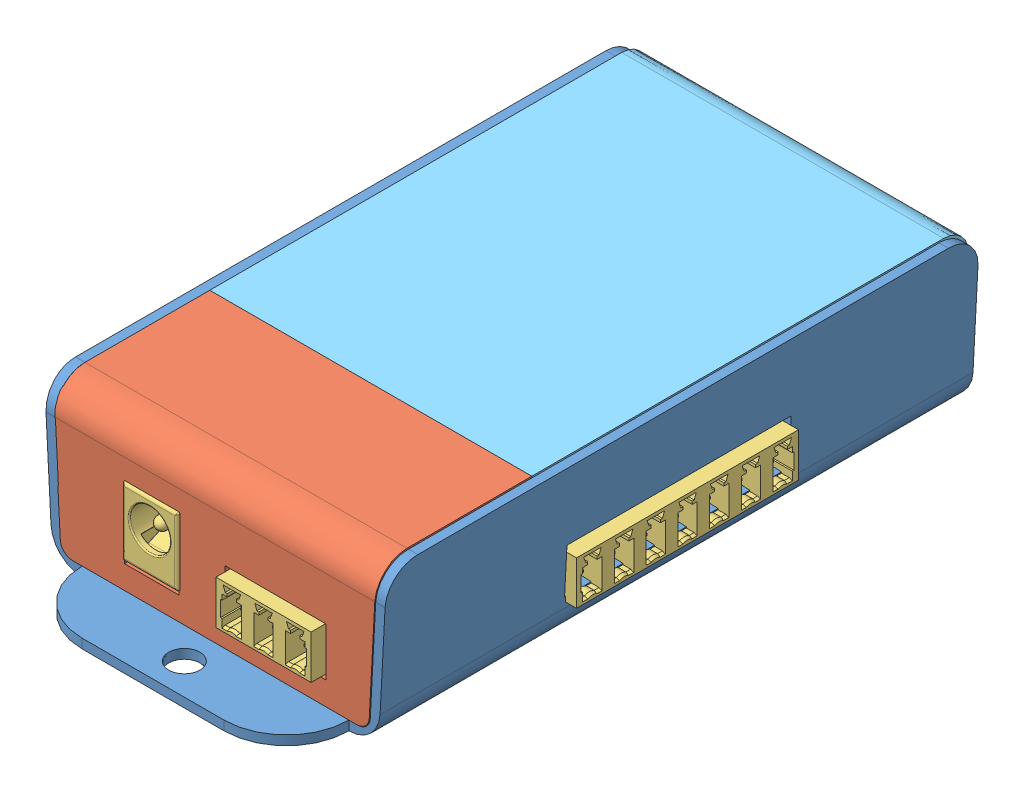
SolidWorks assembly Assembly, configuration Default. Lengths in mm.
Overall size (55.61 25 115).
5 component instances, 5 part files, 12 mates.
Components (placement in the parent):
- Bottom-1: Bottom [Default] at origin size (54.85 25 115)
- top-1: top [Default] at (-0.1229 1.5 47.5) size (51.6 23.5 95)
- PCB2-1: PCB2 [Default] at (-97.96 5.5908 139.76) x (1 0 0) z (0 1 0) size (52.69 93.37 14.6)
- sim7000g-1: sim7000g [Default] at (-18.53 16.5908 34.335) x (0 0 1) z (0 1 0) size (38 37 13.34)
- TOP COVER-1: TOP COVER [Default] at (-25.9229 1.5 47.5029) x (0 0 -1) z (1 0 0) size (72 21.61 51.6)
Mates (geometry in assembly coordinates):
- Coincident1: coordinate: point of Bottom-1; point of assembly
- Coincident2: coincident anti-aligned: plane of Bottom-1 through (-18.5 4 21.5) normal (0 1 0); plane of PCB2-1 through (0 4 50.4369) normal (0 -1 0)
- Concentric1: concentric aligned: cylinder of Bottom-1 through (-18.5 11.4 21.5) axis (0 -1 0) radius 2.2; cylinder of PCB2-1 through (-18.5 4 21.5) axis (0 -1 0) radius 2.5
- Concentric2: concentric aligned: cylinder of Bottom-1 through (18.5 11.4 73.5) axis (0 -1 0) radius 2.2; cylinder of PCB2-1 through (18.5 4 73.5) axis (0 -1 0) radius 2.5
- Coincident12: coincident aligned: line of Bottom-1 through (-22.7934 1.5 95) axis (1 0 0); line of top-1 through (-22.8771 1.5 95) axis (1 0 0)
- Coincident13: coincident aligned: line of Bottom-1 through (-25.9229 25 5) axis (0 0 1); line of top-1 through (-25.9229 25 70) axis (0 0 1)
- Distance1: distance = 11 mm anti-aligned: plane of sim7000g-1 through (-0.03 16.5908 52.835) normal (0 -1 0); plane of PCB2-1 through (0 5.5908 50.4369) normal (0 1 0)
- Parallel5: parallel aligned: plane of PCB2-1 through (-8.23 8.8908 34.7229) normal (-1 0 0); plane of sim7000g-1 through (-18.53 16.5908 34.335) normal (-1 0 0)
- Concentric4: concentric anti-aligned: cylinder of PCB2-1 through (7.59 4 36.535) axis (0 -1 0) radius 0.51; cylinder of sim7000g-1 through (7.59 15.7908 36.535) axis (0 1 0) radius 0.5
- Coincident16: coincident anti-aligned: plane of top-1 through (-30.3229 23.9986 4.8954) normal (0 1 0); plane of TOP COVER-1 through (25.6771 23.9986 4.8983) normal (0 -1 0)
- Coincident17: coincident anti-aligned: plane of top-1 through (-30.3229 25 70) normal (0 0 -1); plane of TOP COVER-1 through (25.6771 25 70) normal (0 0 1)
- Coincident18: coincident aligned: line of Bottom-1 through (-25.9229 25 5) axis (0 0 1); line of TOP COVER-1 through (-25.9229 25 4) axis (0 0 1)
